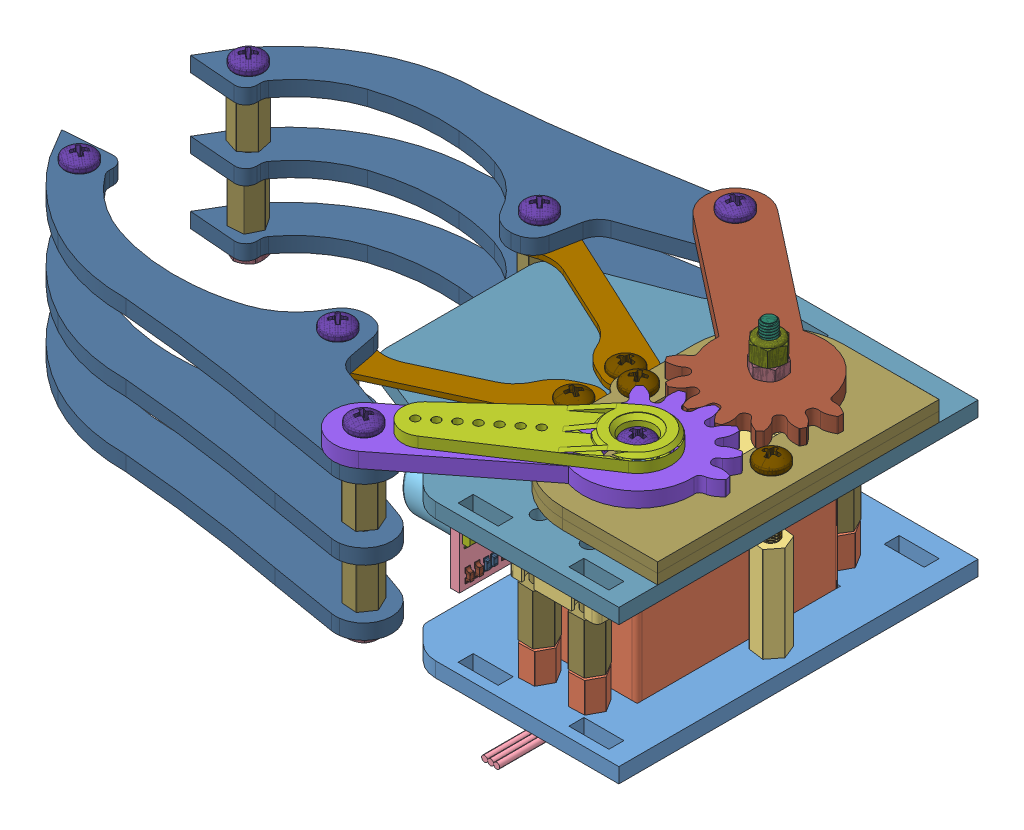
SolidWorks assembly Hand ASM - Gripper, configuration Default. Lengths in mm.
Overall size (134.55 54.17 98.88).
132 component instances, 31 part files, 0 mates.
Components (placement in the parent):
- Hand ASM - Grip.iam-1: Hand ASM - Grip.iam [Default] at origin size (134.55 133.2 98.88)
  - TOWER PRO MG-995, ANALOG SERVO.iam-1: TOWER PRO MG-995, ANALOG SERVO.iam [Default] at (0.0014 -38.65 -10.3) x (-1 0 -0.000132) z (0.000132 0 -1) size (19.82 44.18 67)
    - TOWER PRO MG-995, ANALOG SERVO, BODY, BOTTOM.ipt-1: TOWER PRO MG-995, ANALOG SERVO, BODY, BOTTOM.ipt [Default] at origin size (19.82 6.4 40.62)
    - TOWER PRO MG-995, ANALOG SERVO, BODY, MIDDLE.ipt-1: TOWER PRO MG-995, ANALOG SERVO, BODY, MIDDLE.ipt [Default] at (0 10.25 0) size (19.8 20.5 40.6)
    - TOWER PRO MG-995, ANALOG SERVO, BODY, TOP.ipt-1: TOWER PRO MG-995, ANALOG SERVO, BODY, TOP.ipt [Default] at (0 20.5 0) size (19.8 13.2 54.6)
    - TOWER PRO MG-995, ANALOG SERVO, CONNECTOR.ipt-1: TOWER PRO MG-995, ANALOG SERVO, CONNECTOR.ipt [Default] at (0 -1.3147 -20.3) size (6.8 4.1 19.4)
    - TOWER PRO MG-995, ANALOG SERVO, SHAFT.ipt-1: TOWER PRO MG-995, ANALOG SERVO, SHAFT.ipt [Default] at (0 20.2 -10.3) x (-0.587305 0 -0.809365) z (0.809365 0 -0.587305) size (5.76 17.2 5.8)
    - pan cross head_am_B18.6.7M - M2 x 0.4 x 10 Type I Cross Recessed PHMS --10N.ipt-1: pan cross head_am_B18.6.7M - M2 x 0.4 x 10 Type I Cross Recessed PHMS --10N.ipt [Default] at (-7.7 -6.5 18.1) x (0 1 0) z (0 0 1) size (11.58 4 4)
    - pan cross head_am_B18.6.7M - M2 x 0.4 x 10 Type I Cross Recessed PHMS --10N.ipt-2: pan cross head_am_B18.6.7M - M2 x 0.4 x 10 Type I Cross Recessed PHMS --10N.ipt [Default] at (7.7 -6.5 18.1) x (0 1 0) z (0 0 1) size (11.58 4 4)
    - pan cross head_am_B18.6.7M - M2 x 0.4 x 10 Type I Cross Recessed PHMS --10N.ipt-3: pan cross head_am_B18.6.7M - M2 x 0.4 x 10 Type I Cross Recessed PHMS --10N.ipt [Default] at (7.7 -6.5 -18.1) x (0 1 0) z (0 0 1) size (11.58 4 4)
    - pan cross head_am_B18.6.7M - M2 x 0.4 x 10 Type I Cross Recessed PHMS --10N.ipt-4: pan cross head_am_B18.6.7M - M2 x 0.4 x 10 Type I Cross Recessed PHMS --10N.ipt [Default] at (-7.7 -6.5 -18.1) x (0 1 0) z (0 0 1) size (11.58 4 4)
  - ser Horn.ipt-1: ser Horn.ipt [Default] at (0 -4.8 0) x (0.615661 0 0.788011) z (-0.788011 0 0.615661) size (13.3 7.9 41.35)
  - gearb2a.ipt-1: gearb2a.ipt [Default] x (-0.615661 0 -0.788011) z (0 1 0) size (25.78 59.88 3)
  - arm1b.ipt-1: arm1b.ipt [Default] at (-20.7 -6 -18.315) x (-0.421179 0 0.906978) z (0 -1 0) size (9 45 1)
  - arm1b.ipt-2: arm1b.ipt [Default] at (-20.7 -7 -7.915) x (-0.421186 0 -0.906974) z (0 1 0) size (9 45 1)
  - claw2.ipt-1: claw2.ipt [Default] at (-35.255 -6 -47.2276) x (0.007021 0 0.999975) z (-0.999975 0 0.007021) size (30.05 3 90.37)
  - claw2.ipt-2: claw2.ipt [Default] at (-35.2548 -3 20.9978) x (0.007019 0 -0.999975) z (-0.999975 0 -0.007019) size (30.05 3 90.37)
  - claw2.ipt-3: claw2.ipt [Default] at (-35.255 -20 -47.2276) x (0.007021 0 0.999975) z (-0.999975 0 0.007021) size (30.05 3 90.37)
  - claw2.ipt-4: claw2.ipt [Default] at (-35.255 -33 -47.2276) x (0.007021 0 0.999975) z (-0.999975 0 0.007021) size (30.05 3 90.37)
  - claw2.ipt-5: claw2.ipt [Default] at (-35.2548 -17 20.9978) x (0.007019 0 -0.999975) z (-0.999975 0 -0.007019) size (30.05 3 90.37)
  - claw2.ipt-6: claw2.ipt [Default] at (-35.2548 -30 20.9978) x (0.007019 0 -0.999975) z (-0.999975 0 -0.007019) size (30.05 3 90.37)
  - gearb2b.ipt-1: gearb2b.ipt [Default] at (0 -3 -26.23) x (0.615656 0 -0.788015) z (0 -1 0) size (25.78 59.65 3.01)
  - spacer 10mm.ipt-1: spacer 10mm.ipt [Default] at (-52.8977 -17 -33.2669) x (-0.233974 0 0.972243) z (0 1 0) size (5.5 6.33 16.4)
  - spacer 10mm.ipt-2: spacer 10mm.ipt [Default] at (-52.8976 -17 7.0371) x (0.045425 0 0.998968) z (0 1 0) size (5.5 6.33 16.4)
  - spacer 10mm.ipt-3: spacer 10mm.ipt [Default] at (-30.7324 -16 24.0108) x (-0.809411 0 -0.587242) z (0 1 0) size (5.5 6.33 16.4)
  - spacer 10mm.ipt-4: spacer 10mm.ipt [Default] at (-30.7326 -16 -50.2406) x (0.953387 0 0.301751) z (0 1 0) size (5.5 6.33 16.4)
  - spacer 10mm.ipt-5: spacer 10mm.ipt [Default] at (-52.8977 -30 -33.2669) x (0.333189 0 0.94286) z (0 1 0) size (5.5 6.33 16.4)
  - spacer 10mm.ipt-6: spacer 10mm.ipt [Default] at (-30.7326 -30 -50.2406) x (0.972281 0 -0.233815) z (0 1 0) size (5.5 6.33 16.4)
  - spacer 10mm.ipt-7: spacer 10mm.ipt [Default] at (-30.7324 -30 24.0108) x (-0.900285 0 0.435301) z (0 1 0) size (5.5 6.33 16.4)
  - spacer 10mm.ipt-8: spacer 10mm.ipt [Default] at (-52.8976 -30 7.0371) x (-0.982969 0 -0.183769) z (0 1 0) size (5.5 6.33 16.4)
  - spacer 10mm.ipt-9: spacer 10mm.ipt [Default] at (5.0046 -18.15 -35.189) x (0.841892 0 0.539646) z (0 -1 0) size (5.5 6.33 16.4)
  - spacer 10mm.ipt-10: spacer 10mm.ipt [Default] at (-4.9954 -18.15 -35.1903) x (0.233318 0 0.972401) z (0 -1 0) size (5.5 6.33 16.4)
  - spacer 10mm.ipt-11: spacer 10mm.ipt [Default] at (4.9981 -18.15 14.5903) x (0.01551 0 0.99988) z (0 -1 0) size (5.5 6.33 16.4)
  - spacer 10mm.ipt-12: spacer 10mm.ipt [Default] at (-5.0019 -18.15 14.589) x (0.841892 0 0.539646) z (0 -1 0) size (5.5 6.33 16.4)
  - spacer 10mm.ipt-13: spacer 10mm.ipt [Default] at (-107.8132 -16 -29.9928) x (-0.30966 0 0.950847) z (0 1 0) size (5.5 6.33 16.4)
  - spacer 10mm.ipt-14: spacer 10mm.ipt [Default] at (-107.8131 -16 3.7631) x (-0.143761 0 0.989612) z (0 1 0) size (5.5 6.33 16.4)
  - spacer 10mm.ipt-15: spacer 10mm.ipt [Default] at (-107.8131 -30 3.7631) x (-0.221105 0 0.97525) z (0 1 0) size (5.5 6.33 16.4)
  - spacer 10mm.ipt-16: spacer 10mm.ipt [Default] at (-107.8132 -30 -29.9928) x (0.064998 0 0.997885) z (0 1 0) size (5.5 6.33 16.4)
  - Nut90591A121.ipt-1: Nut90591A121.ipt [Default] at (0 1.2 -26.23) x (-0.497491 0 0.867469) z (0 -1 0) size (7.57 7.57 2.45)
  - Nut90591A121.ipt-2: Nut90591A121.ipt [Default] at (4.686 -31.4241 -4.2332) x (-0.757579 0 0.652743) z (0 -1 0) size (7.57 7.57 2.45)
  - Nut90591A121.ipt-3: Nut90591A121.ipt [Default] at (5.0046 -14.15 -35.189) x (-0.757579 0 -0.652743) z (0 1 0) size (7.57 7.57 2.45)
  - Nut90591A121.ipt-4: Nut90591A121.ipt [Default] at (-4.9954 -14.15 -35.1903) x (-0.757579 0 0.652743) z (0 -1 0) size (7.57 7.57 2.45)
  - Nut90591A121.ipt-5: Nut90591A121.ipt [Default] at (4.9981 -14.15 14.5903) x (-0.563078 0 -0.826404) z (0 -1 0) size (7.57 7.57 2.45)
  - Nut90591A121.ipt-6: Nut90591A121.ipt [Default] at (-5.0019 -14.15 14.589) x (-0.757579 0 0.652743) z (0 -1 0) size (7.57 7.57 2.45)
  - Nut90591A121.ipt-7: Nut90591A121.ipt [Default] at (-30.7326 -34.2 -50.2406) x (-0.121905 0 -0.992542) z (0 1 0) size (7.57 7.57 2.45)
  - Nut90591A121.ipt-8: Nut90591A121.ipt [Default] at (-30.7324 -34.2 24.0108) x (0.975772 0 0.21879) z (0 -1 0) size (7.57 7.57 2.45)
  - Nut90591A121.ipt-9: Nut90591A121.ipt [Default] at (-52.8977 -34.2 -33.2669) x (0.034187 0 0.999415) z (0 -1 0) size (7.57 7.57 2.45)
  - Nut90591A121.ipt-10: Nut90591A121.ipt [Default] at (-52.8976 -34.2 7.0371) x (0.638654 0 0.769494) z (0 -1 0) size (7.57 7.57 2.45)
  - Nut90591A121.ipt-11: Nut90591A121.ipt [Default] at (-20.7 -38.75 -7.915) x (-0.375601 0 -0.926782) z (0 1 0) size (7.57 7.57 2.45)
  - Nut90591A121.ipt-12: Nut90591A121.ipt [Default] at (-20.7 -38.75 -18.315) x (-0.375601 0 -0.926782) z (0 1 0) size (7.57 7.57 2.45)
  - Nut90591A121.ipt-13: Nut90591A121.ipt [Default] at (-13 -38.75 -13.115) x (-0.375601 0 -0.926782) z (0 1 0) size (7.57 7.57 2.45)
  - Nut90591A121.ipt-14: Nut90591A121.ipt [Default] at (13.6 -38.75 -13.115) x (-0.375601 0 0.926782) z (0 -1 0) size (7.57 7.57 2.45)
  - Nut90591A121.ipt-15: Nut90591A121.ipt [Default] at (-107.8131 -34.2 3.7631) x (0.439685 0 -0.898152) z (0 1 0) size (7.57 7.57 2.45)
  - Nut90591A121.ipt-16: Nut90591A121.ipt [Default] at (-107.8132 -34.2 -29.9928) x (0.439685 0 -0.898152) z (0 1 0) size (7.57 7.57 2.45)
  - Dock bot2.ipt-1: Dock bot2.ipt [Default] at (-13 -10 -13.115) size (68.14 3 71.75)
  - 14Screw92005A124.ipt-1: 14Screw92005A124.ipt [Default] at (0 9 -26.23) x (0.305812 0 0.952092) z (0 -1 0) size (6 6 16.38)
  - LNut90576A102.ipt-1: LNut90576A102.ipt [Default] at (0 2.4 -26.23) x (0.749194 0 -0.662351) z (0.662351 0 0.749194) size (7.57 4.12 7.57)
  - 10Screw92005A120.ipt-1: 10Screw92005A120.ipt [Default] at (0 -9.95 0) x (1 0 0) z (0 1 0) size (6 6 12.38)
  - 10Screw92005A120.ipt-2: 10Screw92005A120.ipt [Default] at (-30.7324 -10 24.0108) x (-0.874896 0 -0.484312) z (0 1 0) size (6 6 12.38)
  - 10Screw92005A120.ipt-3: 10Screw92005A120.ipt [Default] at (-30.7326 -10 -50.2406) x (-0.365765 0 0.930707) z (0 1 0) size (6 6 12.38)
  - 10Screw92005A120.ipt-4: 10Screw92005A120.ipt [Default] at (-52.8976 -13 7.0371) x (-0.6941 0 0.719879) z (0 1 0) size (6 6 12.38)
  - 10Screw92005A120.ipt-5: 10Screw92005A120.ipt [Default] at (-52.8977 -13 -33.2669) x (-0.691511 0 0.722366) z (0 1 0) size (6 6 12.38)
  - 10Screw92005A120.ipt-6: 10Screw92005A120.ipt [Default] at (4.9981 -27.55 14.5903) x (-0.54338 0 -0.839487) z (0 -1 0) size (6 6 12.38)
  - 10Screw92005A120.ipt-7: 10Screw92005A120.ipt [Default] at (-5.0019 -27.55 14.589) x (-0.54338 0 -0.839487) z (0 -1 0) size (6 6 12.38)
  - 10Screw92005A120.ipt-8: 10Screw92005A120.ipt [Default] at (5.0046 -27.55 -35.189) x (-0.147707 0 -0.989031) z (0 -1 0) size (6 6 12.38)
  - 10Screw92005A120.ipt-9: 10Screw92005A120.ipt [Default] at (-4.9954 -27.55 -35.1903) x (0.932264 0 -0.361779) z (0 -1 0) size (6 6 12.38)
  - 10Screw92005A120.ipt-10: 10Screw92005A120.ipt [Default] at (-107.8132 -13 -29.9928) x (-0.691511 0 0.722366) z (0 1 0) size (6 6 12.38)
  - 10Screw92005A120.ipt-11: 10Screw92005A120.ipt [Default] at (-107.8131 -13 3.7631) x (-0.569613 0 0.821913) z (0 1 0) size (6 6 12.38)
  - 20Screw92005A128.ipt-1: 20Screw92005A128.ipt [Default] at (13.6 -23 -13.115) x (-0.966394 0 0.257067) z (0 1 0) size (7 6 24.43)
  - 20Screw92005A128.ipt-2: 20Screw92005A128.ipt [Default] at (-20.7 -26.8606 -7.915) x (0.893662 0 0.44874) z (0 1 0) size (7 6 24.43)
  - 20Screw92005A128.ipt-3: 20Screw92005A128.ipt [Default] at (-20.7 -26.6867 -18.315) x (0.991447 0 -0.130512) z (0 1 0) size (7 6 24.43)
  - 20Screw92005A128.ipt-4: 20Screw92005A128.ipt [Default] at (-13 -23 -13.115) x (0.836638 0 -0.547756) z (0 1 0) size (7 6 24.43)
  - Dock bot1 V2.ipt-1: Dock bot1 V2.ipt [Default] at (-13 -34.55 -13.115) x (-1 0 -0.000132) z (-0.000132 0 1) size (44.16 3 71.77)
  - spacer 6mm.ipt-1: spacer 6mm.ipt [Default] at (5.0046 -28.55 -35.189) x (-0.033847 0 -0.999427) z (0 -1 0) size (5.5 6.33 12.4)
  - spacer 6mm.ipt-2: spacer 6mm.ipt [Default] at (-4.9954 -28.55 -35.1903) x (-0.495604 0 -0.868548) z (0 -1 0) size (5.5 6.33 12.4)
  - spacer 6mm.ipt-3: spacer 6mm.ipt [Default] at (4.9981 -28.55 14.5903) x (-0.033847 0 -0.999427) z (0 -1 0) size (5.5 6.33 12.4)
  - spacer 6mm.ipt-4: spacer 6mm.ipt [Default] at (-5.0019 -28.55 14.589) x (-0.033847 0 -0.999427) z (0 -1 0) size (5.5 6.33 12.4)
  - spacer 19mm.ipt-1: spacer 19mm.ipt [Default] at (-20.7 -34.55 -18.315) x (0.70233 0 -0.711852) z (0 1 0) size (5.5 6.33 25.4)
  - spacer 19mm.ipt-2: spacer 19mm.ipt [Default] at (-20.7 -34.55 -7.915) x (0.991892 0 -0.127084) z (0 1 0) size (5.5 6.33 25.4)
  - spacer 19mm.ipt-3: spacer 19mm.ipt [Default] at (-13 -34.55 -13.115) x (0.991892 0 -0.127084) z (0 1 0) size (5.5 6.33 25.4)
  - spacer 19mm.ipt-4: spacer 19mm.ipt [Default] at (13.6 -34.55 -13.115) x (-0.788829 0 -0.614613) z (0 1 0) size (5.5 6.33 25.4)
  - User Library-HC-SR04.iam-1: User Library-HC-SR04.iam [Default] at (-27.5994 -33.4422 -35.1971) x (0 0 1) z (-1 0 0) size (45 25.18 18.07)
    - User Library-HC-SR04_HC-SR04 Ping Sensor.iam-1: User Library-HC-SR04_HC-SR04 Ping Sensor.iam [Default] at (22.5 10.25 -1.75) x (0 -1 0) z (0 0 1) size (25.18 45 18.07)
      - User Library-HC-SR04_PCB.ipt-1: User Library-HC-SR04_PCB.ipt [Default] at origin size (20.53 45 1.75)
      - User Library-HC-SR04_Transducer.ipt-1: User Library-HC-SR04_Transducer.ipt [Default] at (0 -13.16 13.25) x (1 0 0) z (0 -1 0) size (15.88 12 15.88)
      - User Library-HC-SR04_Transducer.ipt-2: User Library-HC-SR04_Transducer.ipt [Default] at (0 12.34 13.25) x (1 0 0) z (0 -1 0) size (15.88 12 15.88)
      - User Library-HC-SR04_3 Pin Header 90 Degree.ipt-1: User Library-HC-SR04_3 Pin Header 90 Degree.ipt [Default] at (8.4275 0 -1.25) x (-1 0 0) z (0 -1 0) size (8 7.82 10)
      - User Library-HC-SR04_14 Pin SMT.ipt-1: User Library-HC-SR04_14 Pin SMT.ipt [Default] at (0 17.5274 -0.85) x (1 0 0) z (0 1 0) size (6 1.6 8.8)
      - User Library-HC-SR04_14 Pin SMT.ipt-2: User Library-HC-SR04_14 Pin SMT.ipt [Default] at (-0.35 -18.5 -0.85) x (0 -1 0) z (1 0 0) size (6 1.6 8.8)
      - User Library-HC-SR04_14 Pin SMT.ipt-3: User Library-HC-SR04_14 Pin SMT.ipt [Default] at (0 -0.3826 -0.85) x (1 0 0) z (0 1 0) size (6 1.6 8.8)
      - User Library-HC-SR04_HC-SR04 Crystal.ipt-1: User Library-HC-SR04_HC-SR04 Crystal.ipt [Default] at (-8.3 0 1.75) x (0 -1 0) z (0 0 1) size (10 3.5 2.7)
      - User Library-HC-SR04_ssot3.ipt-1: User Library-HC-SR04_ssot3.ipt [Default] at (-7.9706 11.2297 0) x (1 0 0) z (0 1 0) size (3 1.13 3.09)
      - User Library-HC-SR04_ssot3.ipt-2: User Library-HC-SR04_ssot3.ipt [Default] at (-7.9706 -14.2327 0) x (1 0 0) z (0 1 0) size (3 1.13 3.09)
      - User Library-HC-SR04_MLC0603.ipt-1: User Library-HC-SR04_MLC0603.ipt [Default] at (7.7901 17.1702 0) x (1 0 0) z (0 1 0) size (2.36 0.6 1.02)
      - User Library-HC-SR04_MLC0603.ipt-2: User Library-HC-SR04_MLC0603.ipt [Default] at (4.9221 -0.625 0) x (0 1 0) z (-1 0 0) size (2.36 0.6 1.02)
      - User Library-HC-SR04_MLC0603.ipt-3: User Library-HC-SR04_MLC0603.ipt [Default] at (-5.1303 17.0114 0) x (0 1 0) z (-1 0 0) size (2.36 0.6 1.02)
      - User Library-HC-SR04_MLC0603.ipt-4: User Library-HC-SR04_MLC0603.ipt [Default] at (-6.3425 7.0242 0) x (0 1 0) z (-1 0 0) size (2.36 0.6 1.02)
      - User Library-HC-SR04_MLC0603.ipt-5: User Library-HC-SR04_MLC0603.ipt [Default] at (-8.2323 14.696 0) x (1 0 0) z (0 1 0) size (2.36 0.6 1.02)
      - User Library-HC-SR04_MLC0603.ipt-6: User Library-HC-SR04_MLC0603.ipt [Default] at (-4.7079 -6.8438 0) x (1 0 0) z (0 1 0) size (2.36 0.6 1.02)
      - User Library-HC-SR04_MLC0603.ipt-7: User Library-HC-SR04_MLC0603.ipt [Default] at (7.5824 9.9685 0) x (1 0 0) z (0 1 0) size (2.36 0.6 1.02)
      - User Library-HC-SR04_MLC0603.ipt-8: User Library-HC-SR04_MLC0603.ipt [Default] at (-8.4554 -9.9341 0) x (0 1 0) z (-1 0 0) size (2.36 0.6 1.02)
      - User Library-HC-SR04_MLC0603.ipt-9: User Library-HC-SR04_MLC0603.ipt [Default] at (-5.0505 19.9858 0) x (0 1 0) z (-1 0 0) size (2.36 0.6 1.02)
      - User Library-HC-SR04_MLC0603.ipt-10: User Library-HC-SR04_MLC0603.ipt [Default] at (0.771 7.4861 0) x (0 1 0) z (-1 0 0) size (2.36 0.6 1.02)
      - User Library-HC-SR04_MLC0603.ipt-11: User Library-HC-SR04_MLC0603.ipt [Default] at (-8.1718 18.0917 0) x (1 0 0) z (0 1 0) size (2.36 0.6 1.02)
      - User Library-HC-SR04_MLC0603.ipt-12: User Library-HC-SR04_MLC0603.ipt [Default] at (7.7433 15.7761 0) x (1 0 0) z (0 1 0) size (2.36 0.6 1.02)
      - User Library-HC-SR04_MLC0603.ipt-13: User Library-HC-SR04_MLC0603.ipt [Default] at (-2.0926 7.3723 0) x (1 0 0) z (0 1 0) size (2.36 0.6 1.02)
      - User Library-HC-SR04_MLC0603.ipt-14: User Library-HC-SR04_MLC0603.ipt [Default] at (-8.2266 4.8481 0) x (1 0 0) z (0 1 0) size (2.36 0.6 1.02)
      - User Library-HC-SR04_MLC0603.ipt-15: User Library-HC-SR04_MLC0603.ipt [Default] at (4.867 -3.8906 0) x (0 1 0) z (-1 0 0) size (2.36 0.6 1.02)
      - User Library-HC-SR04_MLC0603.ipt-16: User Library-HC-SR04_MLC0603.ipt [Default] at (-5.1791 14.6881 0) x (1 0 0) z (0 1 0) size (2.36 0.6 1.02)
      - User Library-HC-SR04_MLC0603.ipt-17: User Library-HC-SR04_MLC0603.ipt [Default] at (-4.2399 7.0151 0) x (0 1 0) z (-1 0 0) size (2.36 0.6 1.02)
      - User Library-HC-SR04_MLC0603.ipt-18: User Library-HC-SR04_MLC0603.ipt [Default] at (-8.2128 13.4796 0) x (1 0 0) z (0 1 0) size (2.36 0.6 1.02)
      - User Library-HC-SR04_MLC0603.ipt-19: User Library-HC-SR04_MLC0603.ipt [Default] at (1.5086 11.2209 0) x (1 0 0) z (0 1 0) size (2.36 0.6 1.02)
      - User Library-HC-SR04_MLC0603.ipt-20: User Library-HC-SR04_MLC0603.ipt [Default] at (-8.276 3.0726 0) x (1 0 0) z (0 1 0) size (2.36 0.6 1.02)
      - User Library-HC-SR04_603 cap on pad.ipt-1: User Library-HC-SR04_603 cap on pad.ipt [Default] at (-7.8553 -18.6213 0) x (1 0 0) z (0 1 0) size (2.76 0.9 1.02)
      - User Library-HC-SR04_603 cap on pad.ipt-2: User Library-HC-SR04_603 cap on pad.ipt [Default] at (2.5708 7.5761 0) x (0 1 0) z (-1 0 0) size (2.76 0.9 1.02)
      - User Library-HC-SR04_603 cap on pad.ipt-3: User Library-HC-SR04_603 cap on pad.ipt [Default] at (-1.0221 -11.2109 0) x (0 1 0) z (-1 0 0) size (2.76 0.9 1.02)
      - User Library-HC-SR04_603 cap on pad.ipt-4: User Library-HC-SR04_603 cap on pad.ipt [Default] at (5.7718 -17.5016 0) x (0 1 0) z (-1 0 0) size (2.76 0.9 1.02)
      - User Library-HC-SR04_603 cap on pad.ipt-5: User Library-HC-SR04_603 cap on pad.ipt [Default] at (-8.0142 0.0287 0) x (1 0 0) z (0 1 0) size (2.76 0.9 1.02)
      - User Library-HC-SR04_603 cap on pad.ipt-6: User Library-HC-SR04_603 cap on pad.ipt [Default] at (7.8006 20.8278 0) x (1 0 0) z (0 1 0) size (2.76 0.9 1.02)
      - User Library-HC-SR04_603 cap on pad.ipt-7: User Library-HC-SR04_603 cap on pad.ipt [Default] at (8.2921 12.7142 0) x (0 1 0) z (-1 0 0) size (2.76 0.9 1.02)
      - User Library-HC-SR04_603 cap on pad.ipt-8: User Library-HC-SR04_603 cap on pad.ipt [Default] at (7.8006 18.9728 0) x (1 0 0) z (0 1 0) size (2.76 0.9 1.02)
      - User Library-HC-SR04_603 cap on pad.ipt-9: User Library-HC-SR04_603 cap on pad.ipt [Default] at (-2.0106 11.2331 0) x (1 0 0) z (0 1 0) size (2.76 0.9 1.02)
      - User Library-HC-SR04_603 cap on pad.ipt-10: User Library-HC-SR04_603 cap on pad.ipt [Default] at (-2.0811 9.4105 0) x (1 0 0) z (0 1 0) size (2.76 0.9 1.02)
      - User Library-HC-SR04_603 cap on pad.ipt-11: User Library-HC-SR04_603 cap on pad.ipt [Default] at (4.491 7.5361 0) x (0 1 0) z (-1 0 0) size (2.76 0.9 1.02)
      - User Library-HC-SR04_603 cap on pad.ipt-12: User Library-HC-SR04_603 cap on pad.ipt [Default] at (0.9766 -11.2109 0) x (0 1 0) z (-1 0 0) size (2.76 0.9 1.02)
      - User Library-HC-SR04_603 cap on pad.ipt-13: User Library-HC-SR04_603 cap on pad.ipt [Default] at (-7.8611 -20.9225 0) x (1 0 0) z (0 1 0) size (2.76 0.9 1.02)
      - User Library-HC-SR04_603 cap on pad.ipt-14: User Library-HC-SR04_603 cap on pad.ipt [Default] at (-8.071 -5.768 0) x (1 0 0) z (0 1 0) size (2.76 0.9 1.02)
      - User Library-HC-SR04_603 cap on pad.ipt-15: User Library-HC-SR04_603 cap on pad.ipt [Default] at (-1.0582 -6.7842 0) x (1 0 0) z (0 1 0) size (2.76 0.9 1.02)
      - User Library-HC-SR04_603 cap on pad.ipt-16: User Library-HC-SR04_603 cap on pad.ipt [Default] at (-8.1408 16.1462 0) x (1 0 0) z (0 1 0) size (2.76 0.9 1.02)
  - Dock top2 V2.ipt-1: Dock top2 V2.ipt [Default] at (0 -7 -26.23) x (0 0 -1) z (1 0 0) size (56.23 2 35.99)
  - Dock top2 V2.ipt-2: Dock top2 V2.ipt [Default] at (0 -5 -26.23) x (0 0 -1) z (1 0 0) size (56.23 2 35.99)
  - Can1.ipt-1: Can1.ipt [Default] at (-80.693 -96.7 -12.966) size (53 133.2 53) (hidden)
